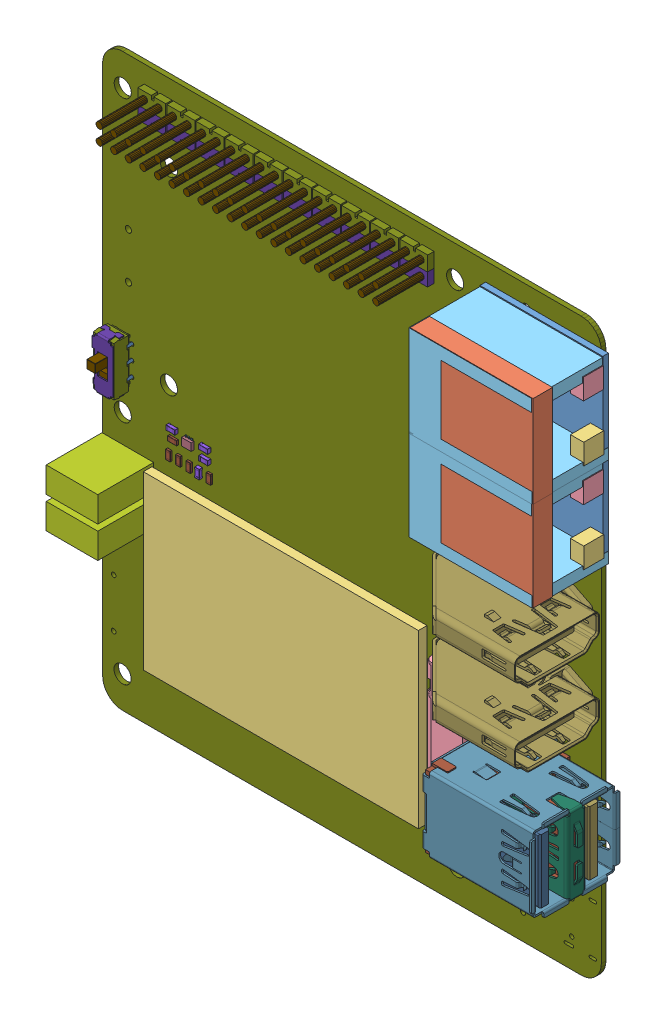
SolidWorks assembly CM4-DUAL-ETH-4G 5G-BASE, configuration Default. Lengths in mm.
Overall size (91.94 99.62 20.53).
748 component instances, 88 part files, 0 mates.
Components (placement in the parent):
- CM4-DUAL-ETH-4G 5G-BASE.step-1: CM4-DUAL-ETH-4G 5G-BASE.step [Default] at origin size (91.94 99.62 20.53)
  - RJ1.step-1: RJ1.step [Default] at origin size (21.67 31.81 13.4)
    - 1103519632.step-1: 1103519632.step [Default] at (77.5484 -26.8671 0) size (21.44 15.98 1)
      - Extruded.step-1: Extruded.step [Default] at origin size (21.44 15.98 1)
    - 1103519760.step-1: 1103519760.step [Default] at (77.7643 -26.9433 10) size (21.46 15.98 3.4)
      - Extruded-0.step-1: Extruded-0.step [Default] at origin size (21.46 15.98 3.4)
    - 1314035072.step-1: 1314035072.step [Default] at (87.2916 -31.8201 1) size (2.34 3.63 3.5)
      - Extruded-1.step-1: Extruded-1.step [Default] at origin size (2.34 3.63 3.5)
    - 1314034944.step-1: 1314034944.step [Default] at (87.2408 -22.0157 1) size (2.34 3.63 3.5)
      - Extruded-2.step-1: Extruded-2.step [Default] at origin size (2.34 3.63 3.5)
    - 1314034816.step-1: 1314034816.step [Default] at (77.5611 -27.0322 0) size (21.46 15.95 13.4)
      - Extruded-3.step-1: Extruded-3.step [Default] at origin size (21.46 15.95 13.4)
    - 1314034816.step-2: 1314034816.step [Default] at (77.5611 -11.3472 0) size (21.46 15.95 13.4)
      - Extruded-3.step-1: Extruded-3.step [Default] at origin size (21.46 15.95 13.4)
    - 1314034944.step-2: 1314034944.step [Default] at (87.2408 -6.3307 1) size (2.34 3.63 3.5)
      - Extruded-2.step-1: Extruded-2.step [Default] at origin size (2.34 3.63 3.5)
    - 1314035072.step-2: 1314035072.step [Default] at (87.2916 -16.1351 1) size (2.34 3.63 3.5)
      - Extruded-1.step-1: Extruded-1.step [Default] at origin size (2.34 3.63 3.5)
    - 1103519760.step-2: 1103519760.step [Default] at (77.7643 -11.2583 10) size (21.46 15.98 3.4)
      - Extruded-0.step-1: Extruded-0.step [Default] at origin size (21.46 15.98 3.4)
    - 1103519632.step-2: 1103519632.step [Default] at (77.5484 -11.1821 0) size (21.44 15.98 1)
      - Extruded.step-1: Extruded.step [Default] at origin size (21.44 15.98 1)
  - R22.step-1: R22.step [Default] at origin size (1.65 0.85 0.46)
    - 575261968.step-1: 575261968.step [Default] at (69.9209 -91.4091 -1.2484) size (1.5 0.8 0.42)
      - Extruded-4.step-1: Extruded-4.step [Default] at origin size (1.5 0.8 0.42)
    - 575262096.step-1: 575262096.step [Default] at (70.6067 -91.4091 -1.2584) size (0.28 0.85 0.46)
      - Extruded-5.step-1: Extruded-5.step [Default] at origin size (0.28 0.85 0.46)
    - 575262096.step-2: 575262096.step [Default] at (69.2352 -91.4091 -1.2584) size (0.28 0.85 0.46)
      - Extruded-5.step-1: Extruded-5.step [Default] at origin size (0.28 0.85 0.46)
  - C2.step-1: C2.step [Default] at origin size (0.8 1.6 0.6)
    - CAPC1608(0603).step-1: CAPC1608(0603).step [Default] at (10.7694 -94.4916 -0.7984) x (0 -1 0) z (0 0 -1) size (1.6 0.8 0.6)
  - H7.step-1: H7.step [Default] at origin size (2.72 1.27 0.46)
    - 663598704.step-1: 663598704.step [Default] at (28.6963 -17.3457 -1.2484) size (2.29 1.12 0.42)
      - Extruded-6.step-1: Extruded-6.step [Default] at origin size (2.29 1.12 0.42)
    - 663598832.step-1: 663598832.step [Default] at (29.9768 -17.3457 -1.2584) size (0.28 1.27 0.46)
      - Extruded-7.step-1: Extruded-7.step [Default] at origin size (0.28 1.27 0.46)
    - 663598832.step-2: 663598832.step [Default] at (27.5279 -17.3457 -1.2584) size (0.28 1.27 0.46)
      - Extruded-7.step-1: Extruded-7.step [Default] at origin size (0.28 1.27 0.46)
  - R78.step-1: R78.step [Default] at origin size (1.65 0.85 0.46)
    - 575262096.step-1: 575262096.step [Default] at (63.7794 -84.0995 -1.2584) size (0.28 0.85 0.46)
      - Extruded-5.step-1: Extruded-5.step [Default] at origin size (0.28 0.85 0.46)
    - 575262096.step-2: 575262096.step [Default] at (62.4079 -84.0995 -1.2584) size (0.28 0.85 0.46)
      - Extruded-5.step-1: Extruded-5.step [Default] at origin size (0.28 0.85 0.46)
    - 575261968.step-1: 575261968.step [Default] at (63.0937 -84.0995 -1.2484) size (1.5 0.8 0.42)
      - Extruded-4.step-1: Extruded-4.step [Default] at origin size (1.5 0.8 0.42)
  - R39.step-1: R39.step [Default] at origin size (1.6 0.8 0.38)
    - RESC1608(0603).step-1: RESC1608(0603).step [Default] at (39.6845 -17.034 -0.7984) x (-1 0 0) z (0 -1 0) size (1.6 0.38 0.8)
  - R37.step-1: R37.step [Default] at origin size (1.6 0.8 0.38)
    - RESC1608(0603).step-1: RESC1608(0603).step [Default] at (39.6845 -15.3114 -0.7984) x (-1 0 0) z (0 -1 0) size (1.6 0.38 0.8)
  - R5.step-1: R5.step [Default] at origin size (1.6 0.8 0.38)
    - RESC1608(0603).step-1: RESC1608(0603).step [Default] at (39.8309 -21.4628 -0.7984) x (-1 0 0) z (0 -1 0) size (1.6 0.38 0.8)
  - R2.step-1: R2.step [Default] at origin size (1.6 0.8 0.38)
    - RESC1608(0603).step-1: RESC1608(0603).step [Default] at (39.8309 -24.5524 -0.7984) x (-1 0 0) z (0 -1 0) size (1.6 0.38 0.8)
  - R1.step-1: R1.step [Default] at origin size (1.6 0.8 0.38)
    - RESC1608(0603).step-1: RESC1608(0603).step [Default] at (39.8309 -23.0076 -0.7984) x (-1 0 0) z (0 -1 0) size (1.6 0.38 0.8)
  - H1.step-1: H1.step [Default] at origin size (1.6 0.8 0.38)
    - RESC1608(0603).step-1: RESC1608(0603).step [Default] at (30.6262 -13.3161 -0.7984) x (-1 0 0) z (0 -1 0) size (1.6 0.38 0.8)
  - H5.step-1: H5.step [Default] at origin size (1.6 0.8 0.38)
    - RESC1608(0603).step-1: RESC1608(0603).step [Default] at (30.6093 -24.1026 -0.7984) x (-1 0 0) z (0 -1 0) size (1.6 0.38 0.8)
  - H6.step-1: H6.step [Default] at origin size (1.6 0.8 0.38)
    - RESC1608(0603).step-1: RESC1608(0603).step [Default] at (30.6093 -21.9377 -0.7984) x (-1 0 0) z (0 -1 0) size (1.6 0.38 0.8)
  - R36.step-1: R36.step [Default] at origin size (1.6 0.8 0.38)
    - RESC1608(0603).step-1: RESC1608(0603).step [Default] at (39.6845 -13.5888 -0.7984) x (-1 0 0) z (0 -1 0) size (1.6 0.38 0.8)
  - HDMI1.step-1: HDMI1.step [Default] at origin size (23.1 7.88 20.15)
    - 72r3759_2007435-1.step-1: 72r3759_2007435-1.step [Default] at (88.2992 -43.8926 9) x (0 1 0) z (1 0 0) size (7.88 20.15 23.1)
  - U14.step-1: U14.step [Default] at origin size (1.7 1.81 0.55)
    - 1348844240.step-1: 1348844240.step [Default] at (15.1262 -53.2966 0.045) size (1.7 1.3 0.5)
      - Extruded-8.step-1: Extruded-8.step [Default] at origin size (1.7 1.3 0.5)
    - 764368800.step-1: 764368800.step [Default] at (15.6262 -52.5945 0) size (0.23 0.4 0.16)
      - Extruded-9.step-1: Extruded-9.step [Default] at origin size (0.23 0.4 0.16)
    - 764368800.step-2: 764368800.step [Default] at (15.1263 -52.5945 0) size (0.23 0.4 0.16)
      - Extruded-9.step-1: Extruded-9.step [Default] at origin size (0.23 0.4 0.16)
    - 764368800.step-3: 764368800.step [Default] at (14.6263 -52.5945 0) size (0.23 0.4 0.16)
      - Extruded-9.step-1: Extruded-9.step [Default] at origin size (0.23 0.4 0.16)
    - 764368800.step-4: 764368800.step [Default] at (14.6263 -53.9965 0) size (0.23 0.4 0.16)
      - Extruded-9.step-1: Extruded-9.step [Default] at origin size (0.23 0.4 0.16)
    - 764368800.step-5: 764368800.step [Default] at (15.1263 -53.9965 0) size (0.23 0.4 0.16)
      - Extruded-9.step-1: Extruded-9.step [Default] at origin size (0.23 0.4 0.16)
    - 764368800.step-6: 764368800.step [Default] at (15.6263 -53.9965 0) size (0.23 0.4 0.16)
      - Extruded-9.step-1: Extruded-9.step [Default] at origin size (0.23 0.4 0.16)
  - R73.step-1: R73.step [Default] at origin size (0.8 1.6 0.38)
    - RESC1608(0603).step-1: RESC1608(0603).step [Default] at (13.494 -56.6964 0) x (0 1 0) z (1 0 0) size (1.6 0.38 0.8)
  - R72.step-1: R72.step [Default] at origin size (0.8 1.6 0.38)
    - RESC1608(0603).step-1: RESC1608(0603).step [Default] at (15.2725 -56.7662 0) x (0 -1 0) z (-1 0 0) size (1.6 0.38 0.8)
  - R71.step-1: R71.step [Default] at origin size (0.8 1.6 0.38)
    - RESC1608(0603).step-1: RESC1608(0603).step [Default] at (11.7419 -56.7662 0) x (0 -1 0) z (-1 0 0) size (1.6 0.38 0.8)
  - R70.step-1: R70.step [Default] at origin size (0.8 1.6 0.38)
    - RESC1608(0603).step-1: RESC1608(0603).step [Default] at (18.8031 -56.7662 0) x (0 -1 0) z (-1 0 0) size (1.6 0.38 0.8)
  - R69.step-1: R69.step [Default] at origin size (1.6 0.8 0.38)
    - RESC1608(0603).step-1: RESC1608(0603).step [Default] at (12.4687 -54.179 0) x (1 0 0) z (0 -1 0) size (1.6 0.38 0.8)
  - L7.step-1: L7.step [Default] at origin size (6.5 7.2 2.9)
    - 1127965152.step-1: 1127965152.step [Default] at (17.9746 -48.1322 -3.7984) size (6.5 7.2 2.9)
      - Extruded-10.step-1: Extruded-10.step [Default] at origin size (6.5 7.2 2.9)
  - KEY1.step-1: KEY1.step [Default] at origin size (3.6 9 8.45)
    - User_Library-MMP221.step-1: User_Library-MMP221.step [Default] at (3.4634 -45.8936 0) x (0 1 0) z (1 0 0) size (9 8.45 3.6)
      - User_Library-MMP221_MMP221.step-1: User_Library-MMP221_MMP221.step [Default] at (0 3.3 0) x (-1 0 0) z (0 0 1) size (8.9 3.3 3.6)
      - User_Library-MMP221_MMP221_SM.step-1: User_Library-MMP221_MMP221_SM.step [Default] at (0 3.3 0) x (-1 0 0) z (0 0 -1) size (9 2.1 3.6)
      - User_Library-MMP221_MMP221_PP.step-1: User_Library-MMP221_MMP221_PP.step [Default] at (1 1.2 0) x (-1 0 0) z (0 0 -1) size (6 4.3 2.6)
      - User_Library-MMP221_MMP221_PIN.step-1: User_Library-MMP221_MMP221_PIN.step [Default] at (0 1.05 0) size (0.6 4 3.2)
      - User_Library-MMP221_MMP221_PIN.step-2: User_Library-MMP221_MMP221_PIN.step [Default] at (2.5 1.05 0) size (0.6 4 3.2)
      - User_Library-MMP221_MMP221_PIN.step-3: User_Library-MMP221_MMP221_PIN.step [Default] at (-2.5 1.05 0) size (0.6 4 3.2)
  - C102.step-1: C102.step [Default] at origin size (1.6 0.8 0.6)
    - CAPC1608(0603).step-1: CAPC1608(0603).step [Default] at (19.7102 -43.0166 -0.7984) x (-1 0 0) z (0 0 -1) size (1.6 0.8 0.6)
  - C101.step-1: C101.step [Default] at origin size (1.6 0.8 0.6)
    - CAPC1608(0603).step-1: CAPC1608(0603).step [Default] at (16.3525 -43.0371 -0.7984) x (1 0 0) z (0 0 -1) size (1.6 0.8 0.6)
  - C100.step-1: C100.step [Default] at origin size (0.8 1.6 0.6)
    - CAPC1608(0603).step-1: CAPC1608(0603).step [Default] at (17.0311 -56.7181 0) x (0 1 0) z (0 0 1) size (1.6 0.8 0.6)
  - C99.step-1: C99.step [Default] at origin size (1.6 0.8 0.6)
    - CAPC1608(0603).step-1: CAPC1608(0603).step [Default] at (18.1108 -54.2618 0) x (1 0 0) z (0 0 1) size (1.6 0.8 0.6)
  - C98.step-1: C98.step [Default] at origin size (1.6 0.8 0.6)
    - CAPC1608(0603).step-1: CAPC1608(0603).step [Default] at (18.0852 -52.5347 0) x (-1 0 0) z (0 0 1) size (1.6 0.8 0.6)
  - C97.step-1: C97.step [Default] at origin size (1.6 0.8 0.6)
    - CAPC1608(0603).step-1: CAPC1608(0603).step [Default] at (12.3956 -52.4839 0) x (-1 0 0) z (0 0 1) size (1.6 0.8 0.6)
  - TVS1.step-1: TVS1.step [Default] at origin size (2.26 2 1.05)
    - User_Library-SOT-363.step-1: User_Library-SOT-363.step [Default] at (18.2037 -82.092 0) x (0 -1 0) z (0 0 1) size (2 2.26 1.05)
  - SIMCOM1.step-1: SIMCOM1.step [Default] at origin size (56.01 29.97 4.02)
    - 663597680.step-1: 663597680.step [Default] at (34.593 -73.1988 2) size (48.01 29.97 1.5)
      - Extruded-11.step-1: Extruded-11.step [Default] at origin size (48.01 29.97 1.5)
    - 89w2147_2199119-3.step-1: 89w2147_2199119-3.step [Default] at (58.246 -73.1627 1.8) x (0 -1 0) z (-1 0 0) size (21.9 3.7 8.7)
  - R65.step-1: R65.step [Default] at origin size (1.6 0.8 0.38)
    - RESC1608(0603).step-1: RESC1608(0603).step [Default] at (18.2734 -80.3285 0) x (1 0 0) z (0 -1 0) size (1.6 0.38 0.8)
  - R63.step-1: R63.step [Default] at origin size (1.6 0.8 0.38)
    - RESC1608(0603).step-1: RESC1608(0603).step [Default] at (18.2734 -83.8424 0) x (1 0 0) z (0 -1 0) size (1.6 0.38 0.8)
  - R62.step-1: R62.step [Default] at origin size (1.6 0.8 0.38)
    - RESC1608(0603).step-1: RESC1608(0603).step [Default] at (18.2036 -85.6126 0) x (-1 0 0) z (0 1 0) size (1.6 0.38 0.8)
  - R61.step-1: R61.step [Default] at origin size (1.6 0.8 0.38)
    - RESC1608(0603).step-1: RESC1608(0603).step [Default] at (52.8513 -64.7592 0) x (1 0 0) z (0 -1 0) size (1.6 0.38 0.8)
  - R60.step-1: R60.step [Default] at origin size (1.6 0.8 0.38)
    - RESC1608(0603).step-1: RESC1608(0603).step [Default] at (10.7955 -82.0987 0) x (-1 0 0) z (0 1 0) size (1.6 0.38 0.8)
  - R59.step-1: R59.step [Default] at origin size (1.6 0.8 0.38)
    - RESC1608(0603).step-1: RESC1608(0603).step [Default] at (10.7955 -80.3417 0) x (-1 0 0) z (0 1 0) size (1.6 0.38 0.8)
  - R58.step-1: R58.step [Default] at origin size (1.6 0.8 0.38)
    - RESC1608(0603).step-1: RESC1608(0603).step [Default] at (52.7894 -81.5725 0) x (-1 0 0) z (0 1 0) size (1.6 0.38 0.8)
  - R54.step-1: R54.step [Default] at origin size (1.6 0.8 0.38)
    - RESC1608(0603).step-1: RESC1608(0603).step [Default] at (52.8617 -73.2495 0) x (1 0 0) z (0 -1 0) size (1.6 0.38 0.8)
  - R53.step-1: R53.step [Default] at origin size (1.6 0.8 0.38)
    - RESC1608(0603).step-1: RESC1608(0603).step [Default] at (52.8592 -79.9158 0) x (1 0 0) z (0 -1 0) size (1.6 0.38 0.8)
  - R52.step-1: R52.step [Default] at origin size (1.6 0.8 0.38)
    - RESC1608(0603).step-1: RESC1608(0603).step [Default] at (52.7894 -74.8236 0) x (-1 0 0) z (0 1 0) size (1.6 0.38 0.8)
  - R51.step-1: R51.step [Default] at origin size (1.6 0.8 0.38)
    - RESC1608(0603).step-1: RESC1608(0603).step [Default] at (52.7894 -71.7017 0) x (-1 0 0) z (0 1 0) size (1.6 0.38 0.8)
  - R50.step-1: R50.step [Default] at origin size (1.6 0.8 0.38)
    - RESC1608(0603).step-1: RESC1608(0603).step [Default] at (52.7894 -70.1694 0) x (-1 0 0) z (0 1 0) size (1.6 0.38 0.8)
  - Q7.step-1: Q7.step [Default] at origin size (2.64 3 1.08)
    - ALSRobot-SOT23.step-1: ALSRobot-SOT23.step [Default] at (52.8095 -67.5135 0) x (0 -1 0) z (0 0 1) size (3 2.64 1.08)
  - Q6.step-1: Q6.step [Default] at origin size (2.64 3 1.08)
    - ALSRobot-SOT23.step-1: ALSRobot-SOT23.step [Default] at (52.8174 -77.2017 0) x (0 -1 0) z (0 0 1) size (3 2.64 1.08)
  - L4.step-1: L4.step [Default] at origin size (9.95 4.45 11.5)
    - 1015527712.step-1: 1015527712.step [Default] at (0.9405 -66.9019 3) x (0 -1 0) z (0 0 1) size (3.5 3.5 3.5)
      - Sphere.step-1: Sphere.step [Default] at origin size (3.5 3.5 3.5)
    - 1103520528.step-1: 1103520528.step [Default] at (4.6411 -66.9011 0.254) size (9 4.45 9.75)
      - Extruded-12.step-1: Extruded-12.step [Default] at origin size (9 4.45 9.75)
    - 1015527832.step-1: 1015527832.step [Default] at (0.9405 -66.9019 8) x (0 -1 0) z (0 0 1) size (3.5 3.5 3.5)
      - Sphere-13.step-1: Sphere-13.step [Default] at origin size (3.5 3.5 3.5)
    - 1015527952.step-1: 1015527952.step [Default] at (7.7605 -65.6318 -1.5) x (0 1 0) z (0 0 1) size (0.76 0.76 5)
      - Cylinder.step-1: Cylinder.step [Default] at origin size (0.76 0.76 5)
    - 1015527952.step-2: 1015527952.step [Default] at (5.2205 -65.6318 -1.5) x (0 1 0) z (0 0 1) size (0.76 0.76 5)
      - Cylinder.step-1: Cylinder.step [Default] at origin size (0.76 0.76 5)
    - 1015527952.step-3: 1015527952.step [Default] at (5.2205 -68.1718 -1.5) x (0 1 0) z (0 0 1) size (0.76 0.76 5)
      - Cylinder.step-1: Cylinder.step [Default] at origin size (0.76 0.76 5)
    - 1015527952.step-4: 1015527952.step [Default] at (7.7605 -68.1718 -1.5) x (0 1 0) z (0 0 1) size (0.76 0.76 5)
      - Cylinder.step-1: Cylinder.step [Default] at origin size (0.76 0.76 5)
  - C94.step-1: C94.step [Default] at origin size (1.6 0.8 0.6)
    - CAPC1608(0603).step-1: CAPC1608(0603).step [Default] at (14.7077 -80.335 0) x (1 0 0) z (0 0 1) size (1.6 0.8 0.6)
  - C92.step-1: C92.step [Default] at origin size (1.6 0.8 0.6)
    - CAPC1608(0603).step-1: CAPC1608(0603).step [Default] at (14.7077 -85.6059 0) x (1 0 0) z (0 0 1) size (1.6 0.8 0.6)
  - C91.step-1: C91.step [Default] at origin size (1.6 0.8 0.6)
    - CAPC1608(0603).step-1: CAPC1608(0603).step [Default] at (14.7077 -82.092 0) x (1 0 0) z (0 0 1) size (1.6 0.8 0.6)
  - C90.step-1: C90.step [Default] at origin size (0.8 1.6 0.6)
    - CAPC1608(0603).step-1: CAPC1608(0603).step [Default] at (45.5624 -61.984 0) x (0 1 0) z (0 0 1) size (1.6 0.8 0.6)
  - C89.step-1: C89.step [Default] at origin size (0.8 1.6 0.6)
    - CAPC1608(0603).step-1: CAPC1608(0603).step [Default] at (44.0637 -61.984 0) x (0 1 0) z (0 0 1) size (1.6 0.8 0.6)
  - C88.step-1: C88.step [Default] at origin size (0.8 1.6 0.6)
    - CAPC1608(0603).step-1: CAPC1608(0603).step [Default] at (77.2669 -88.5749 -0.7984) x (0 1 0) z (0 0 -1) size (1.6 0.8 0.6)
  - J1.step-1: J1.step [Default] at origin size (20.5 15.59 19.61)
    - 44000.step-1: 44000.step [Default] at (72.6815 -73.7566 7.8016) x (-1 0 0) z (0 0 -1) size (20.5 15.59 19.61)
      - SOLID.step-1: SOLID.step [Default] at origin size (19.25 11.1 2.6)
      - SOLID-14.step-1: SOLID-14.step [Default] at origin size (19.3 13.3 15.01)
      - SOLID-15.step-1: SOLID-15.step [Default] at origin size (19.25 11.1 2.6)
      - SOLID-16.step-1: SOLID-16.step [Default] at origin size (5.49 11.5 14.69)
      - SOLID-17.step-1: SOLID-17.step [Default] at origin size (18.21 1.45 17.25)
      - SOLID-18.step-1: SOLID-18.step [Default] at origin size (18.21 1.45 17.25)
      - SOLID-19.step-1: SOLID-19.step [Default] at origin size (18.21 1.45 17.25)
      - SOLID-20.step-1: SOLID-20.step [Default] at origin size (18.21 1.45 17.25)
      - SOLID-21.step-1: SOLID-21.step [Default] at origin size (18.21 1.45 17.25)
      - SOLID-22.step-1: SOLID-22.step [Default] at origin size (12.91 1 15.85)
      - SOLID-23.step-1: SOLID-23.step [Default] at origin size (12.91 1 15.85)
      - SOLID-24.step-1: SOLID-24.step [Default] at origin size (12.91 1 15.81)
      - SOLID-25.step-1: SOLID-25.step [Default] at origin size (12.91 1 15.81)
      - SOLID-26.step-1: SOLID-26.step [Default] at origin size (15.01 1.45 8.75)
      - SOLID-27.step-1: SOLID-27.step [Default] at origin size (15.01 1.45 8.75)
      - SOLID-28.step-1: SOLID-28.step [Default] at origin size (15.01 1.45 8.75)
      - SOLID-29.step-1: SOLID-29.step [Default] at origin size (15.01 1.45 8.75)
      - SOLID-30.step-1: SOLID-30.step [Default] at origin size (15.01 1.45 8.75)
      - SOLID-31.step-1: SOLID-31.step [Default] at origin size (10.42 1 7.35)
      - SOLID-32.step-1: SOLID-32.step [Default] at origin size (10.42 1 7.35)
      - SOLID-33.step-1: SOLID-33.step [Default] at origin size (10.42 1 7.35)
      - SOLID-34.step-1: SOLID-34.step [Default] at origin size (10.42 1 7.35)
      - SOLID-35.step-1: SOLID-35.step [Default] at origin size (19.7 15.59 19.61)
      - SOLID-36.step-1: SOLID-36.step [Default] at origin size (16.1 13.62 4.38)
  - PI1.step-1: PI1.step [Default] at origin size (50.58 4.88 11.2)
    - 1466328752.step-1: 1466328752.step [Default] at (9.6693 -4.3696 0) size (4.86 2.63 1.1)
      - Extruded-37.step-1: Extruded-37.step [Default] at origin size (4.86 2.63 1.1)
    - 1503596240.step-1: 1503596240.step [Default] at (9.6693 -6.7686 0) size (4.86 2.33 1.1)
      - Extruded-38.step-1: Extruded-38.step [Default] at origin size (4.86 2.33 1.1)
    - 1503596240.step-2: 1503596240.step [Default] at (14.7493 -6.7686 0) size (4.86 2.33 1.1)
      - Extruded-38.step-1: Extruded-38.step [Default] at origin size (4.86 2.33 1.1)
    - 1466328752.step-2: 1466328752.step [Default] at (14.7493 -4.3696 0) size (4.86 2.63 1.1)
      - Extruded-37.step-1: Extruded-37.step [Default] at origin size (4.86 2.63 1.1)
    - 1503596240.step-3: 1503596240.step [Default] at (19.8293 -6.7686 0) size (4.86 2.33 1.1)
      - Extruded-38.step-1: Extruded-38.step [Default] at origin size (4.86 2.33 1.1)
    - 1466328752.step-3: 1466328752.step [Default] at (19.8293 -4.3696 0) size (4.86 2.63 1.1)
      - Extruded-37.step-1: Extruded-37.step [Default] at origin size (4.86 2.63 1.1)
    - 1503596240.step-4: 1503596240.step [Default] at (24.9093 -6.7686 0) size (4.86 2.33 1.1)
      - Extruded-38.step-1: Extruded-38.step [Default] at origin size (4.86 2.33 1.1)
    - 1466328752.step-4: 1466328752.step [Default] at (24.9093 -4.3696 0) size (4.86 2.63 1.1)
      - Extruded-37.step-1: Extruded-37.step [Default] at origin size (4.86 2.63 1.1)
    - 1503596240.step-5: 1503596240.step [Default] at (29.9893 -6.7686 0) size (4.86 2.33 1.1)
      - Extruded-38.step-1: Extruded-38.step [Default] at origin size (4.86 2.33 1.1)
    - 1466328752.step-5: 1466328752.step [Default] at (29.9893 -4.3696 0) size (4.86 2.63 1.1)
      - Extruded-37.step-1: Extruded-37.step [Default] at origin size (4.86 2.63 1.1)
    - 1503596240.step-6: 1503596240.step [Default] at (35.0693 -6.7686 0) size (4.86 2.33 1.1)
      - Extruded-38.step-1: Extruded-38.step [Default] at origin size (4.86 2.33 1.1)
    - 1466328752.step-6: 1466328752.step [Default] at (35.0693 -4.3696 0) size (4.86 2.63 1.1)
      - Extruded-37.step-1: Extruded-37.step [Default] at origin size (4.86 2.63 1.1)
    - 1503596240.step-7: 1503596240.step [Default] at (40.1493 -6.7686 0) size (4.86 2.33 1.1)
      - Extruded-38.step-1: Extruded-38.step [Default] at origin size (4.86 2.33 1.1)
    - 1466328752.step-7: 1466328752.step [Default] at (40.1493 -4.3696 0) size (4.86 2.63 1.1)
      - Extruded-37.step-1: Extruded-37.step [Default] at origin size (4.86 2.63 1.1)
    - 1503596240.step-8: 1503596240.step [Default] at (45.2293 -6.7686 0) size (4.86 2.33 1.1)
      - Extruded-38.step-1: Extruded-38.step [Default] at origin size (4.86 2.33 1.1)
    - 1466328752.step-8: 1466328752.step [Default] at (45.2293 -4.3696 0) size (4.86 2.63 1.1)
      - Extruded-37.step-1: Extruded-37.step [Default] at origin size (4.86 2.63 1.1)
    - 1503596240.step-9: 1503596240.step [Default] at (50.3093 -6.7686 0) size (4.86 2.33 1.1)
      - Extruded-38.step-1: Extruded-38.step [Default] at origin size (4.86 2.33 1.1)
    - 1466328752.step-9: 1466328752.step [Default] at (50.3093 -4.3696 0) size (4.86 2.63 1.1)
      - Extruded-37.step-1: Extruded-37.step [Default] at origin size (4.86 2.63 1.1)
    - 1503596240.step-10: 1503596240.step [Default] at (55.3893 -6.7686 0) size (4.86 2.33 1.1)
      - Extruded-38.step-1: Extruded-38.step [Default] at origin size (4.86 2.33 1.1)
    - 1466328752.step-10: 1466328752.step [Default] at (55.3893 -4.3696 0) size (4.86 2.63 1.1)
      - Extruded-37.step-1: Extruded-37.step [Default] at origin size (4.86 2.63 1.1)
    - 1466328880.step-1: 1466328880.step [Default] at (8.3884 -6.781 -2.2) size (1.11 1.11 11.2)
      - Extruded-39.step-1: Extruded-39.step [Default] at origin size (1.11 1.11 11.2)
    - 1466328880.step-2: 1466328880.step [Default] at (8.3884 -4.241 -2.2) size (1.11 1.11 11.2)
      - Extruded-39.step-1: Extruded-39.step [Default] at origin size (1.11 1.11 11.2)
    - 1466328880.step-3: 1466328880.step [Default] at (10.9285 -6.781 -2.2) size (1.11 1.11 11.2)
      - Extruded-39.step-1: Extruded-39.step [Default] at origin size (1.11 1.11 11.2)
    - 1466328880.step-4: 1466328880.step [Default] at (10.9285 -4.241 -2.2) size (1.11 1.11 11.2)
      - Extruded-39.step-1: Extruded-39.step [Default] at origin size (1.11 1.11 11.2)
    - 1466328880.step-5: 1466328880.step [Default] at (13.4685 -6.781 -2.2) size (1.11 1.11 11.2)
      - Extruded-39.step-1: Extruded-39.step [Default] at origin size (1.11 1.11 11.2)
    - 1466328880.step-6: 1466328880.step [Default] at (13.4685 -4.241 -2.2) size (1.11 1.11 11.2)
      - Extruded-39.step-1: Extruded-39.step [Default] at origin size (1.11 1.11 11.2)
    - 1466328880.step-7: 1466328880.step [Default] at (16.0085 -6.781 -2.2) size (1.11 1.11 11.2)
      - Extruded-39.step-1: Extruded-39.step [Default] at origin size (1.11 1.11 11.2)
    - 1466328880.step-8: 1466328880.step [Default] at (16.0085 -4.241 -2.2) size (1.11 1.11 11.2)
      - Extruded-39.step-1: Extruded-39.step [Default] at origin size (1.11 1.11 11.2)
    - 1466328880.step-9: 1466328880.step [Default] at (18.5484 -6.781 -2.2) size (1.11 1.11 11.2)
      - Extruded-39.step-1: Extruded-39.step [Default] at origin size (1.11 1.11 11.2)
    - 1466328880.step-10: 1466328880.step [Default] at (18.5484 -4.241 -2.2) size (1.11 1.11 11.2)
      - Extruded-39.step-1: Extruded-39.step [Default] at origin size (1.11 1.11 11.2)
    - 1466328880.step-11: 1466328880.step [Default] at (21.0885 -6.781 -2.2) size (1.11 1.11 11.2)
      - Extruded-39.step-1: Extruded-39.step [Default] at origin size (1.11 1.11 11.2)
    - 1466328880.step-12: 1466328880.step [Default] at (21.0885 -4.241 -2.2) size (1.11 1.11 11.2)
      - Extruded-39.step-1: Extruded-39.step [Default] at origin size (1.11 1.11 11.2)
    - 1466328880.step-13: 1466328880.step [Default] at (23.6285 -6.781 -2.2) size (1.11 1.11 11.2)
      - Extruded-39.step-1: Extruded-39.step [Default] at origin size (1.11 1.11 11.2)
    - 1466328880.step-14: 1466328880.step [Default] at (23.6285 -4.241 -2.2) size (1.11 1.11 11.2)
      - Extruded-39.step-1: Extruded-39.step [Default] at origin size (1.11 1.11 11.2)
    - 1466328880.step-15: 1466328880.step [Default] at (26.1685 -6.781 -2.2) size (1.11 1.11 11.2)
      - Extruded-39.step-1: Extruded-39.step [Default] at origin size (1.11 1.11 11.2)
    - 1466328880.step-16: 1466328880.step [Default] at (26.1685 -4.241 -2.2) size (1.11 1.11 11.2)
      - Extruded-39.step-1: Extruded-39.step [Default] at origin size (1.11 1.11 11.2)
    - 1466328880.step-17: 1466328880.step [Default] at (28.7084 -6.781 -2.2) size (1.11 1.11 11.2)
      - Extruded-39.step-1: Extruded-39.step [Default] at origin size (1.11 1.11 11.2)
    - 1466328880.step-18: 1466328880.step [Default] at (28.7084 -4.241 -2.2) size (1.11 1.11 11.2)
      - Extruded-39.step-1: Extruded-39.step [Default] at origin size (1.11 1.11 11.2)
    - 1466328880.step-19: 1466328880.step [Default] at (31.2485 -6.781 -2.2) size (1.11 1.11 11.2)
      - Extruded-39.step-1: Extruded-39.step [Default] at origin size (1.11 1.11 11.2)
    - 1466328880.step-20: 1466328880.step [Default] at (31.2485 -4.241 -2.2) size (1.11 1.11 11.2)
      - Extruded-39.step-1: Extruded-39.step [Default] at origin size (1.11 1.11 11.2)
    - 1466328880.step-21: 1466328880.step [Default] at (33.7885 -6.781 -2.2) size (1.11 1.11 11.2)
      - Extruded-39.step-1: Extruded-39.step [Default] at origin size (1.11 1.11 11.2)
    - 1466328880.step-22: 1466328880.step [Default] at (33.7885 -4.241 -2.2) size (1.11 1.11 11.2)
      - Extruded-39.step-1: Extruded-39.step [Default] at origin size (1.11 1.11 11.2)
    - 1466328880.step-23: 1466328880.step [Default] at (36.3284 -6.781 -2.2) size (1.11 1.11 11.2)
      - Extruded-39.step-1: Extruded-39.step [Default] at origin size (1.11 1.11 11.2)
    - 1466328880.step-24: 1466328880.step [Default] at (36.3284 -4.241 -2.2) size (1.11 1.11 11.2)
      - Extruded-39.step-1: Extruded-39.step [Default] at origin size (1.11 1.11 11.2)
    - 1466328880.step-25: 1466328880.step [Default] at (38.8685 -6.781 -2.2) size (1.11 1.11 11.2)
      - Extruded-39.step-1: Extruded-39.step [Default] at origin size (1.11 1.11 11.2)
    - 1466328880.step-26: 1466328880.step [Default] at (38.8685 -4.241 -2.2) size (1.11 1.11 11.2)
      - Extruded-39.step-1: Extruded-39.step [Default] at origin size (1.11 1.11 11.2)
    - 1466328880.step-27: 1466328880.step [Default] at (41.4085 -6.781 -2.2) size (1.11 1.11 11.2)
      - Extruded-39.step-1: Extruded-39.step [Default] at origin size (1.11 1.11 11.2)
    - 1466328880.step-28: 1466328880.step [Default] at (41.4085 -4.241 -2.2) size (1.11 1.11 11.2)
      - Extruded-39.step-1: Extruded-39.step [Default] at origin size (1.11 1.11 11.2)
    - 1466328880.step-29: 1466328880.step [Default] at (43.9485 -6.781 -2.2) size (1.11 1.11 11.2)
      - Extruded-39.step-1: Extruded-39.step [Default] at origin size (1.11 1.11 11.2)
    - 1466328880.step-30: 1466328880.step [Default] at (43.9485 -4.241 -2.2) size (1.11 1.11 11.2)
      - Extruded-39.step-1: Extruded-39.step [Default] at origin size (1.11 1.11 11.2)
    - 1466328880.step-31: 1466328880.step [Default] at (46.4884 -6.781 -2.2) size (1.11 1.11 11.2)
      - Extruded-39.step-1: Extruded-39.step [Default] at origin size (1.11 1.11 11.2)
    - 1466328880.step-32: 1466328880.step [Default] at (46.4884 -4.241 -2.2) size (1.11 1.11 11.2)
      - Extruded-39.step-1: Extruded-39.step [Default] at origin size (1.11 1.11 11.2)
    - 1466328880.step-33: 1466328880.step [Default] at (49.0285 -6.781 -2.2) size (1.11 1.11 11.2)
      - Extruded-39.step-1: Extruded-39.step [Default] at origin size (1.11 1.11 11.2)
    - 1466328880.step-34: 1466328880.step [Default] at (49.0285 -4.241 -2.2) size (1.11 1.11 11.2)
      - Extruded-39.step-1: Extruded-39.step [Default] at origin size (1.11 1.11 11.2)
    - 1466328880.step-35: 1466328880.step [Default] at (51.5685 -6.781 -2.2) size (1.11 1.11 11.2)
      - Extruded-39.step-1: Extruded-39.step [Default] at origin size (1.11 1.11 11.2)
    - 1466328880.step-36: 1466328880.step [Default] at (51.5685 -4.241 -2.2) size (1.11 1.11 11.2)
      - Extruded-39.step-1: Extruded-39.step [Default] at origin size (1.11 1.11 11.2)
    - 1466328880.step-37: 1466328880.step [Default] at (54.1084 -6.781 -2.2) size (1.11 1.11 11.2)
      - Extruded-39.step-1: Extruded-39.step [Default] at origin size (1.11 1.11 11.2)
    - 1466328880.step-38: 1466328880.step [Default] at (54.1084 -4.241 -2.2) size (1.11 1.11 11.2)
      - Extruded-39.step-1: Extruded-39.step [Default] at origin size (1.11 1.11 11.2)
    - 1466328880.step-39: 1466328880.step [Default] at (56.6485 -6.781 -2.2) size (1.11 1.11 11.2)
      - Extruded-39.step-1: Extruded-39.step [Default] at origin size (1.11 1.11 11.2)
    - 1466328880.step-40: 1466328880.step [Default] at (56.6485 -4.241 -2.2) size (1.11 1.11 11.2)
      - Extruded-39.step-1: Extruded-39.step [Default] at origin size (1.11 1.11 11.2)
  - R19.step-1: R19.step [Default] at origin size (0.8 1.6 0.38)
    - RESC1608(0603).step-1: RESC1608(0603).step [Default] at (55.2872 -41.4682 -0.7984) x (0 -1 0) z (1 0 0) size (1.6 0.38 0.8)
  - R7.step-1: R7.step [Default] at origin size (0.8 1.6 0.38)
    - RESC1608(0603).step-1: RESC1608(0603).step [Default] at (56.8229 -41.4682 -0.7984) x (0 -1 0) z (1 0 0) size (1.6 0.38 0.8)
  - C85.step-1: C85.step [Default] at origin size (1.6 0.8 0.6)
    - CAPC1608(0603).step-1: CAPC1608(0603).step [Default] at (11.4504 -68.9687 -0.7984) x (1 0 0) z (0 0 -1) size (1.6 0.8 0.6)
  - R42.step-1: R42.step [Default] at origin size (1.6 0.8 0.38)
    - RESC1608(0603).step-1: RESC1608(0603).step [Default] at (20.7078 -68.9867 -0.7984) x (-1 0 0) z (0 -1 0) size (1.6 0.38 0.8)
  - R41.step-1: R41.step [Default] at origin size (1.6 0.8 0.38)
    - RESC1608(0603).step-1: RESC1608(0603).step [Default] at (16.0306 -68.9783 -0.7984) x (-1 0 0) z (0 -1 0) size (1.6 0.38 0.8)
  - L2.step-1: L2.step [Default] at origin size (4.4 4 1.97)
    - 764368672.step-1: 764368672.step [Default] at (12.0725 -60.2189 -2.7984) size (4.4 4 1.97)
      - Extruded-40.step-1: Extruded-40.step [Default] at origin size (4.4 4 1.97)
  - IN1.step-1: IN1.step [Default] at origin size (5.08 2.54 2.29)
    - 880594368.step-1: 880594368.step [Default] at (13.1901 -55.881 -3.0844) size (5.08 2.54 2.29)
      - Extruded-41.step-1: Extruded-41.step [Default] at origin size (5.08 2.54 2.29)
  - C86.step-1: C86.step [Default] at origin size (1.6 0.8 0.6)
    - CAPC1608(0603).step-1: CAPC1608(0603).step [Default] at (20.7558 -65.5584 -0.7984) x (1 0 0) z (0 0 -1) size (1.6 0.8 0.6)
  - C81.step-1: C81.step [Default] at origin size (3.2 1.6 1.1)
    - INDC3216(1206).step-1: INDC3216(1206).step [Default] at (19.7687 -55.8531 -0.7984) x (1 0 0) z (0 1 0) size (3.2 1.1 1.6)
  - Y1.step-1: Y1.step [Default] at origin size (3.95 3.1 1)
    - 1081399232.step-1: 1081399232.step [Default] at (55.2454 -27.8136 -1.7984) size (3.95 3.1 1)
      - Extruded-42.step-1: Extruded-42.step [Default] at origin size (3.95 3.1 1)
  - U6.step-1: U6.step [Default] at origin size (5 5 0.83)
    - 575262992.step-1: 575262992.step [Default] at (57.6658 -34.957 -1.6484) size (5 5 0.83)
      - Extruded-43.step-1: Extruded-43.step [Default] at origin size (5 5 0.83)
  - Y3.step-1: Y3.step [Default] at origin size (3.95 3.1 1)
    - 1081399232.step-1: 1081399232.step [Default] at (43.0933 -80.7653 0) size (3.95 3.1 1)
      - Extruded-42.step-1: Extruded-42.step [Default] at origin size (3.95 3.1 1)
  - U7.step-1: U7.step [Default] at origin size (8.1 8.1 0.83)
    - 880596288.step-1: 880596288.step [Default] at (39.1687 -70.7339 0.02) size (8.1 8.1 0.83)
      - Extruded-44.step-1: Extruded-44.step [Default] at origin size (8.1 8.1 0.83)
  - R31.step-1: R31.step [Default] at origin size (1.6 0.8 0.38)
    - RESC1608(0603).step-1: RESC1608(0603).step [Default] at (29.9452 -67.4397 0) x (1 0 0) z (0 -1 0) size (1.6 0.38 0.8)
  - R29.step-1: R29.step [Default] at origin size (1.6 0.8 0.38)
    - RESC1608(0603).step-1: RESC1608(0603).step [Default] at (51.4841 -34.1268 -0.7984) x (-1 0 0) z (0 -1 0) size (1.6 0.38 0.8)
  - R28.step-1: R28.step [Default] at origin size (0.8 1.6 0.38)
    - RESC1608(0603).step-1: RESC1608(0603).step [Default] at (47.9001 -80.8002 0) x (0 -1 0) z (-1 0 0) size (1.6 0.38 0.8)
  - R27.step-1: R27.step [Default] at origin size (0.8 1.6 0.38)
    - RESC1608(0603).step-1: RESC1608(0603).step [Default] at (49.5511 -80.9018 0) x (0 -1 0) z (-1 0 0) size (1.6 0.38 0.8)
  - R26.step-1: R26.step [Default] at origin size (1.6 0.8 0.38)
    - RESC1608(0603).step-1: RESC1608(0603).step [Default] at (29.8754 -64.5414 0) x (-1 0 0) z (0 1 0) size (1.6 0.38 0.8)
  - R25.step-1: R25.step [Default] at origin size (0.8 1.6 0.38)
    - RESC1608(0603).step-1: RESC1608(0603).step [Default] at (30.9892 -80.8002 0) x (0 -1 0) z (-1 0 0) size (1.6 0.38 0.8)
  - R24.step-1: R24.step [Default] at origin size (0.8 1.6 0.38)
    - RESC1608(0603).step-1: RESC1608(0603).step [Default] at (32.7864 -80.8002 0) x (0 -1 0) z (-1 0 0) size (1.6 0.38 0.8)
  - R23.step-1: R23.step [Default] at origin size (0.8 1.6 0.38)
    - RESC1608(0603).step-1: RESC1608(0603).step [Default] at (34.5836 -80.8002 0) x (0 -1 0) z (-1 0 0) size (1.6 0.38 0.8)
  - R14.step-1: R14.step [Default] at origin size (0.8 1.6 0.38)
    - RESC1608(0603).step-1: RESC1608(0603).step [Default] at (61.4562 -27.9703 -0.7984) x (0 -1 0) z (1 0 0) size (1.6 0.38 0.8)
  - R13.step-1: R13.step [Default] at origin size (0.8 1.6 0.38)
    - RESC1608(0603).step-1: RESC1608(0603).step [Default] at (30.3209 -82.0401 -0.7984) x (0 -1 0) z (1 0 0) size (1.6 0.38 0.8)
  - R9.step-1: R9.step [Default] at origin size (1.6 0.8 0.38)
    - RESC1608(0603).step-1: RESC1608(0603).step [Default] at (29.9452 -71.8069 0) x (1 0 0) z (0 -1 0) size (1.6 0.38 0.8)
  - R4.step-1: R4.step [Default] at origin size (0.8 1.6 0.38)
    - RESC1608(0603).step-1: RESC1608(0603).step [Default] at (50.1808 -77.6632 -0.7984) x (0 1 0) z (-1 0 0) size (1.6 0.38 0.8)
  - R3.step-1: R3.step [Default] at origin size (0.8 1.6 0.38)
    - RESC1608(0603).step-1: RESC1608(0603).step [Default] at (48.3774 -77.6632 -0.7984) x (0 1 0) z (-1 0 0) size (1.6 0.38 0.8)
  - PWR4.step-1: PWR4.step [Default] at origin size (0.8 1.6 0.6)
    - CAPC1608(0603).step-1: CAPC1608(0603).step [Default] at (43.1546 -86.8022 0) x (0 -1 0) z (0 0 1) size (1.6 0.8 0.6)
  - PWR3.step-1: PWR3.step [Default] at origin size (1.6 3.2 1.1)
    - INDC3216(1206).step-1: INDC3216(1206).step [Default] at (40.9804 -86.7891 0) x (0 1 0) z (1 0 0) size (3.2 1.1 1.6)
  - PWR2.step-1: PWR2.step [Default] at origin size (0.8 1.6 0.6)
    - CAPC1608(0603).step-1: CAPC1608(0603).step [Default] at (29.1853 -86.776 0) x (0 1 0) z (0 0 1) size (1.6 0.8 0.6)
  - PWR1.step-1: PWR1.step [Default] at origin size (1.6 3.2 1.1)
    - INDC3216(1206).step-1: INDC3216(1206).step [Default] at (31.2395 -86.7891 0) x (0 -1 0) z (-1 0 0) size (3.2 1.1 1.6)
  - I1.step-1: I1.step [Default] at origin size (2.3 1.2 1.1)
    - User_Library-1N4148WS.step-1: User_Library-1N4148WS.step [Default] at (29.9102 -73.5917 0.2516) x (1 0 0) z (0 0 -1) size (2.3 1.2 1.1)
  - C78.step-1: C78.step [Default] at origin size (1.6 0.8 0.6)
    - CAPC1608(0603).step-1: CAPC1608(0603).step [Default] at (29.9288 -65.9363 0) x (1 0 0) z (0 0 1) size (1.6 0.8 0.6)
  - C77.step-1: C77.step [Default] at origin size (1.6 0.8 0.6)
    - CAPC1608(0603).step-1: CAPC1608(0603).step [Default] at (48.9722 -77.0114 0) x (-1 0 0) z (0 0 1) size (1.6 0.8 0.6)
  - C76.step-1: C76.step [Default] at origin size (1.6 0.8 0.6)
    - CAPC1608(0603).step-1: CAPC1608(0603).step [Default] at (48.9722 -78.443 0) x (-1 0 0) z (0 0 1) size (1.6 0.8 0.6)
  - C73.step-1: C73.step [Default] at origin size (1.6 0.8 0.6)
    - CAPC1608(0603).step-1: CAPC1608(0603).step [Default] at (29.923 -68.902 0) x (1 0 0) z (0 0 1) size (1.6 0.8 0.6)
  - C72.step-1: C72.step [Default] at origin size (0.8 1.6 0.6)
    - CAPC1608(0603).step-1: CAPC1608(0603).step [Default] at (33.6738 -61.99 0) x (0 -1 0) z (0 0 1) size (1.6 0.8 0.6)
  - C71.step-1: C71.step [Default] at origin size (0.8 1.6 0.6)
    - CAPC1608(0603).step-1: CAPC1608(0603).step [Default] at (36.5851 -61.99 0) x (0 -1 0) z (0 0 1) size (1.6 0.8 0.6)
  - C70.step-1: C70.step [Default] at origin size (0.8 1.6 0.6)
    - CAPC1608(0603).step-1: CAPC1608(0603).step [Default] at (38.1714 -80.7526 0) x (0 1 0) z (0 0 1) size (1.6 0.8 0.6)
  - C69.step-1: C69.step [Default] at origin size (0.8 1.6 0.6)
    - CAPC1608(0603).step-1: CAPC1608(0603).step [Default] at (35.1295 -61.99 0) x (0 -1 0) z (0 0 1) size (1.6 0.8 0.6)
  - C68.step-1: C68.step [Default] at origin size (1.6 0.8 0.6)
    - CAPC1608(0603).step-1: CAPC1608(0603).step [Default] at (49.0658 -72.7009 0) x (-1 0 0) z (0 0 1) size (1.6 0.8 0.6)
  - C67.step-1: C67.step [Default] at origin size (0.8 1.6 0.6)
    - CAPC1608(0603).step-1: CAPC1608(0603).step [Default] at (32.2181 -61.9645 0) x (0 1 0) z (0 0 1) size (1.6 0.8 0.6)
  - C66.step-1: C66.step [Default] at origin size (0.8 1.6 0.6)
    - CAPC1608(0603).step-1: CAPC1608(0603).step [Default] at (30.7625 -61.9645 0) x (0 1 0) z (0 0 1) size (1.6 0.8 0.6)
  - C64.step-1: C64.step [Default] at origin size (0.8 1.6 0.6)
    - CAPC1608(0603).step-1: CAPC1608(0603).step [Default] at (29.1853 -80.7526 0) x (0 1 0) z (0 0 1) size (1.6 0.8 0.6)
  - C63.step-1: C63.step [Default] at origin size (1.6 0.8 0.6)
    - CAPC1608(0603).step-1: CAPC1608(0603).step [Default] at (49.0658 -68.3592 0) x (-1 0 0) z (0 0 1) size (1.6 0.8 0.6)
  - C62.step-1: C62.step [Default] at origin size (0.8 1.6 0.6)
    - CAPC1608(0603).step-1: CAPC1608(0603).step [Default] at (29.2118 -61.9258 0) x (0 -1 0) z (0 0 1) size (1.6 0.8 0.6)
  - C61.step-1: C61.step [Default] at origin size (0.8 1.6 0.6)
    - CAPC1608(0603).step-1: CAPC1608(0603).step [Default] at (40.9667 -61.99 0) x (0 -1 0) z (0 0 1) size (1.6 0.8 0.6)
  - C60.step-1: C60.step [Default] at origin size (1.6 0.8 0.6)
    - CAPC1608(0603).step-1: CAPC1608(0603).step [Default] at (29.8967 -78.443 0) x (-1 0 0) z (0 0 1) size (1.6 0.8 0.6)
  - C59.step-1: C59.step [Default] at origin size (0.8 1.6 0.6)
    - CAPC1608(0603).step-1: CAPC1608(0603).step [Default] at (42.4374 -61.99 0) x (0 -1 0) z (0 0 1) size (1.6 0.8 0.6)
  - C57.step-1: C57.step [Default] at origin size (1.6 0.8 0.6)
    - CAPC1608(0603).step-1: CAPC1608(0603).step [Default] at (49.0658 -66.9119 0) x (-1 0 0) z (0 0 1) size (1.6 0.8 0.6)
  - C56.step-1: C56.step [Default] at origin size (1.6 0.8 0.6)
    - CAPC1608(0603).step-1: CAPC1608(0603).step [Default] at (49.0658 -65.4647 0) x (-1 0 0) z (0 0 1) size (1.6 0.8 0.6)
  - C55.step-1: C55.step [Default] at origin size (0.8 1.6 0.6)
    - CAPC1608(0603).step-1: CAPC1608(0603).step [Default] at (64.587 -27.3526 -0.7984) x (0 -1 0) z (0 0 -1) size (1.6 0.8 0.6)
  - C54.step-1: C54.step [Default] at origin size (0.8 1.6 0.6)
    - CAPC1608(0603).step-1: CAPC1608(0603).step [Default] at (46.3694 -80.8542 0) x (0 1 0) z (0 0 1) size (1.6 0.8 0.6)
  - C53.step-1: C53.step [Default] at origin size (0.8 1.6 0.6)
    - CAPC1608(0603).step-1: CAPC1608(0603).step [Default] at (39.9687 -80.7781 0) x (0 -1 0) z (0 0 1) size (1.6 0.8 0.6)
  - C52.step-1: C52.step [Default] at origin size (0.8 1.6 0.6)
    - CAPC1608(0603).step-1: CAPC1608(0603).step [Default] at (58.3654 -41.4202 -0.7984) x (0 1 0) z (0 0 -1) size (1.6 0.8 0.6)
